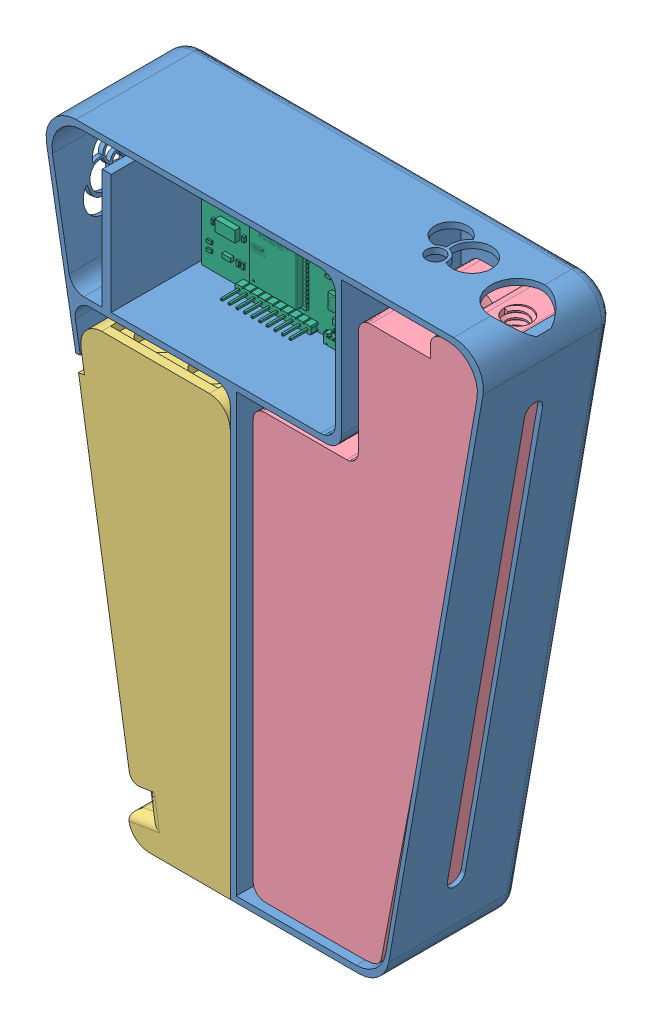
SolidWorks assembly Assembly, configuration Default. Lengths in mm.
Overall size (146.2 200 48.83).
17 component instances, 11 part files, 30 mates.
Components (placement in the parent):
- New_front-1: New_front [Default] at (-4.246 -92.8661 -24.1061) size (146.2 200 43.2)
- Front_Plate_Circles-1: Front_Plate_Circles [Default] at (-3.3346 -89.8378 -24.3635) x (-0.999657 0 -0.026177) z (0.026177 0 -0.999657) size (104.68 126.62 2.01)
- Battery_Box-4: Battery_Box [Default] at (0.8043 0 -21.1061) size (50.72 142.98 40.53)
- BackPlate-3: BackPlate [Default] at (-4.246 -92.8661 21.8939) x (-1 0 0) z (0 0 -1) size (146.2 200 3.01) (hidden)
- New_Water_Comp_Bottom_With-3: New_Water_Comp_Bottom_With [Default] at (-3.1111 -94.3661 -21.1061) size (78.59 193 37)
- Real_Water-1: Real_Water [Default] at (-3.1111 -94.3661 -20.1061) size (61.77 122.02 35)
- PCB1.step-7: PCB1.step [Default] at (-54.2902 55.8029 -10.0891) size (66.55 48.68 11.98)
- Motion_Detector-2: Motion_Detector [Default] at (-140.0018 191.2616 -23.0384) x (0.629105 0.777146 0.016474) z (0.026177 0 -0.999657) size (10.5 10.5 10)
- Cotton_Stick_Small-7: Cotton_Stick_Small [Default] at (-7.234 31.1339 4.476) x (-1 0 0) z (0 0 -1) size (5 8 5)
- Cotton_Stick-7: Cotton_Stick [Default] at (-7.234 -88.8661 4.476) x (-1 0 0) z (0 0 -1) size (5 30 5)
- Cotton_Stick-10: Cotton_Stick [Default] at (-3.3105 45.7147 0.5401) x (0 -0.309017 0.951057) z (0 0.951057 0.309017) size (5 30 5)
- Cotton_Stick-11: Cotton_Stick [Default] at (28.9335 43.2509 2.1519) size (5 30 5)
- Cotton_Stick-12: Cotton_Stick [Default] at (-7.234 -28.8661 4.476) x (-1 0 0) z (0 0 -1) size (5 30 5)
- Cotton_Stick-13: Cotton_Stick [Default] at (-7.234 1.1339 4.476) x (-1 0 0) z (0 0 -1) size (5 30 5)
- Cotton_Stick-14: Cotton_Stick [Default] at (-7.234 -58.8661 4.476) x (-1 0 0) z (0 0 -1) size (5 30 5)
- Cotton_Stick_Small-12: Cotton_Stick_Small [Default] at (-7.234 39.1339 4.476) x (-1 0 0) z (0 0 -1) size (5 8 5)
- Front_Plate_Logo-2: Front_Plate_Logo [Default] at (-16.1834 -116.3267 -23.2482) x (-0.999848 0 0.017452) z (-0.017452 0 -0.999848) size (28.07 9.36 2)
Mates (geometry in assembly coordinates):
- Coincident9: coincident anti-aligned: plane of New_front-1 through (-43.246 -90.8661 18.8939) normal (0.985285 0.170917 0); plane of Battery_Box-3 through (-44.4852 -83.722 18.8939) normal (-0.985285 -0.170917 0)
- Coincident10: coincident anti-aligned: plane of New_front-1 through (-4.246 -92.8661 -21.1061) normal (0 0 1); plane of Battery_Box-3 through (0.8554 0.6932 -21.1061) normal (0 0 -1)
- Coincident21: coincident anti-aligned: line of New_front-1 through (-13.7681 -90.8661 18.8939) axis (0 1 0); line of Sponge-3 through (-13.7681 -69.8661 18.8939) axis (0 -1 0)
- Coincident22: coincident aligned: line of New_front-1 through (58.8521 107.1339 18.8939) axis (-1 0 0); line of BackPlate-2 through (58.8521 107.1339 18.8939) axis (-1 0 0)
- Coincident27: coincident aligned: line of New_front-1 through (68.7024 95.4101 -20.6061) axis (0 0 1); line of BackPlate-2 through (68.7024 95.4101 18.8939) axis (0 0 1)
- Coincident29: coincident anti-aligned: line of New_front-1 through (58.8521 107.1339 18.8939) axis (-1 0 0); line of BackPlate-3 through (-67.344 107.1339 18.8939) axis (1 0 0)
- Coincident30: coincident anti-aligned: line of New_front-1 through (-77.1943 95.4101 18.8939) axis (0.17238 -0.98503 0); line of BackPlate-3 through (-45.6943 -84.5899 18.8939) axis (-0.17238 0.98503 0)
- Coincident34: coincident aligned: line of New_front-1 through (-15.7681 -92.8302 -21.1061) axis (0 1 0); line of Battery_Box-4 through (-15.7681 -92.8661 -21.1061) axis (0 1 0)
- Coincident35: coincident anti-aligned: line of BackPlate-3 through (27.3521 -92.8661 18.8939) axis (-1 0 0); line of Battery_Box-4 through (-42.7681 -92.8661 18.8939) axis (1 0 0)
- Coincident36: coincident aligned: line of New_front-1 through (-13.7681 -90.8661 18.8939) axis (1 0 0); line of New_Water_Comp_Bottom-1 through (-39.1798 -90.8661 18.8939) axis (1 0 0)
- Coincident43: coincident anti-aligned: plane of New_front-1 through (-4.246 -92.8661 -21.1061) normal (0 0 1); plane of New_Water_Comp_Bottom_With-3 through (-3.1111 -94.3661 -21.1061) normal (0 0 -1)
- Coincident48: coincident anti-aligned: plane of New_Water_Comp_Bottom_With-3 through (65.5254 100.1339 -20.1061) normal (-0.981973 0.189022 0); plane of Real_Water-1 through (52.6327 33.1561 14.8939) normal (0.981973 -0.189022 0)
- Coincident49: coincident aligned: line of New_Water_Comp_Bottom_With-3 through (0.8667 -88.8661 -20.1061) axis (1 0 0); line of Real_Water-1 through (-9.1333 -88.8661 -20.1061) axis (1 0 0)
- InPlace1: in place: plane of New_front-1 through (-4.246 -92.8661 -21.1061) normal (0 0 1); plane of ? through (0 0 -21.1061) normal (0 0 1); moOrthogonalPlaneRef_w of New_front-1 through (-4.246 -92.8661 -21.1061) normal (0 0 1); plane of ? through (0 0 -21.1061) normal (0 1 0); plane of New_front-1 through (-4.246 -92.8661 -21.1061) normal (0 0 1); plane of ? through (0 0 -21.1061) normal (1 0 0); plane of New_front-1 through (-4.246 -92.8661 -21.1061) normal (0 0 1); unknown of ?
- Coincident50: coincident aligned: plane of New_front-1; plane of ?
- Coincident51: coincident aligned: moOrthogonalPlaneRef_w of New_front-1 through (-4.246 -92.8661 -21.1061) normal (0 1 0); plane of Part1^Assembly-1 through (-4.246 -92.8661 -21.1061) normal (0 1 0)
- Coincident52: coincident anti-aligned: moOrthogonalPlaneRef_w of New_front-1 through (-4.246 -92.8661 -21.1061) normal (-1 0 0); plane of Part1^Assembly-1 through (-4.246 -92.8661 -21.1061) normal (1 0 0)
- Coincident53: coincident anti-aligned: plane of New_Water_Comp_Bottom_With-3 through (-9.1333 -88.8661 -20.1061) normal (0 1 0); plane of Cotton_Stick-1 through (66.9517 -88.8661 11.2861) normal (0 -1 0)
- Tangent1: tangent anti-aligned: plane of New_Water_Comp_Bottom_With-3 through (-9.1333 48.8907 -20.1061) normal (1 0 0); cylinder of Cotton_Stick-1 through (66.9517 -78.8661 11.2861) axis (0 -1 0) radius 2.5
- Coincident54: coincident anti-aligned: plane of Cotton_Stick-1 through (66.9517 -78.8661 11.2861) normal (0 1 0); plane of Cotton_Stick_Small-6 through (66.9517 -78.8661 11.2861) normal (0 -1 0)
- Coincident55: coincident aligned: circle of Cotton_Stick-1; circle of Cotton_Stick-6
- Coincident56: coincident aligned: circle of Cotton_Stick-5; circle of Cotton_Stick-6
- Coincident57: coincident aligned: circle of Cotton_Stick-4; circle of Cotton_Stick-5
- Coincident60: coincident anti-aligned: plane of New_Water_Comp_Bottom_With-3 through (-9.1333 -88.8661 -20.1061) normal (0 1 0); plane of Cotton_Stick-7 through (-7.234 -88.8661 4.476) normal (0 -1 0)
- Coincident62: coincident aligned: circle of Cotton_Stick-7; circle of Cotton_Stick-14
- Coincident63: coincident aligned: circle of Cotton_Stick-12; circle of Cotton_Stick-14
- Coincident65: coincident aligned: circle of Cotton_Stick-12; circle of Cotton_Stick-13
- Coincident66: coincident aligned: circle of Cotton_Stick_Small-7; circle of Cotton_Stick-13
- Coincident68: coincident aligned: circle of Cotton_Stick_Small-7; circle of Cotton_Stick_Small-12
- Coincident69: coincident aligned: circle of Cotton_Stick_Small-7; circle of Cotton_Stick_Small-12
